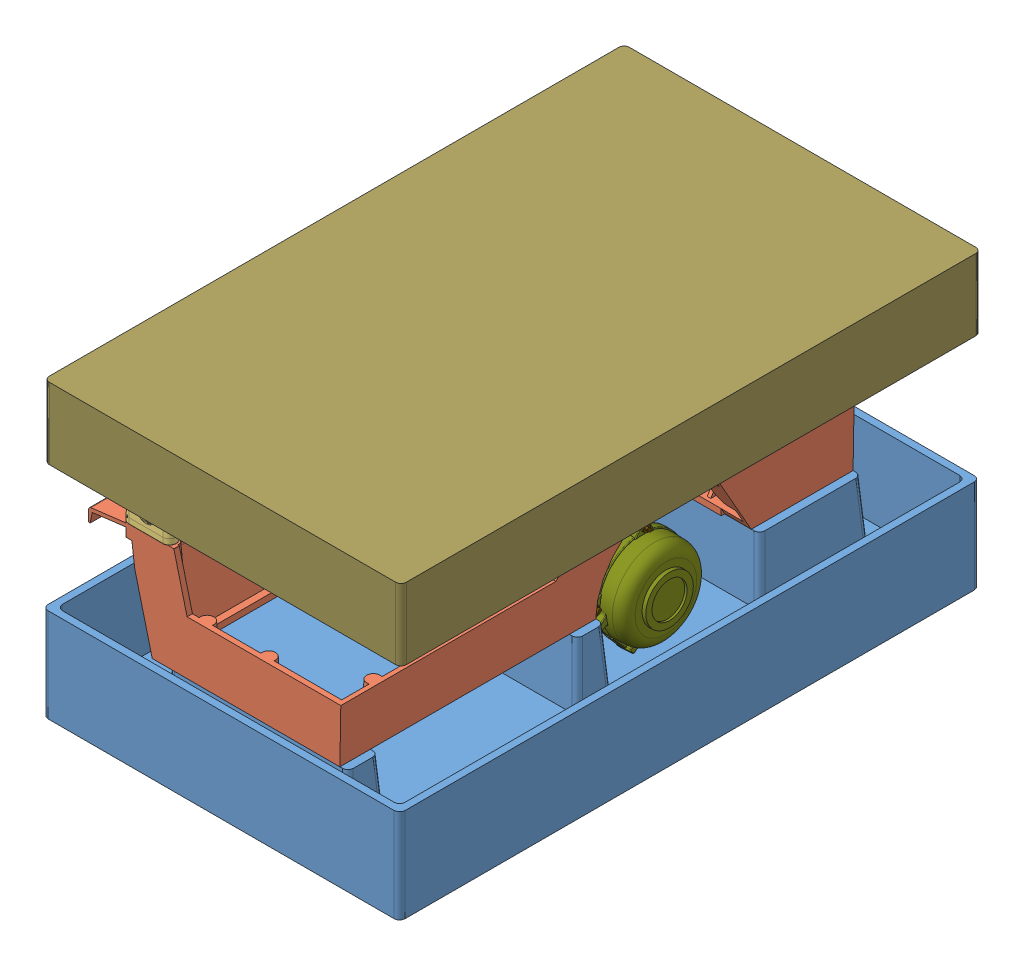
SolidWorks assembly Siège de dentiste, configuration Défaut. Lengths in mm.
Overall size (401 374.1 650.58).
134 component instances, 46 part files, 15 mates.
Components (placement in the parent):
- Chassis-1: Chassis [Défaut] at origin size (400 245.59 650)
  - Base-2: Base [Défaut] at (19.488 0 0) x (1 0 0) z (0 -1 0) size (400 650 105)
  - Chassis-1: Chassis [Défaut] at origin size (284.75 158.03 576.08)
  - Demi-bride-1: Demi-bride [Défaut] at (-215.8786 159.586 270) x (1 0 0) z (0 -1 0) size (53 15 19.91)
  - Demi-bride-2: Demi-bride [Défaut] at (-215.8786 159.586 524) x (-1 0 0) z (0 -1 0) size (53 15 19.91)
  - Demi-bride-3: Demi-bride [Défaut] at (-215.8786 118.686 524) x (1 0 0) z (0 1 0) size (53 15 19.91)
  - Demi-bride-4: Demi-bride [Défaut] at (-215.8786 118.686 270) x (-1 0 0) z (0 1 0) size (53 15 19.91)
  - Axe de guidage-1: Axe de guidage [Défaut] at (-215.8786 139.136 527.5) x (0.966925 -0.255061 0) z (0 0 -1) size (25 25 263)
  - Rondelle plate 5,3-10-1: Rondelle plate 5,3-10 [Défaut] at (-234.8786 160.586 270) x (0 -1 0) z (0 0 1) size (1 10 10)
  - Vis chc M5-50-1: Vis chc M5-50 [Défaut] at (-234.8786 160.586 270) x (0 -1 0) z (0.008588 0 0.999963) size (55 8.5 8.5)
  - Rondelle plate 5,3-10-2: Rondelle plate 5,3-10 [Défaut] at (-234.8786 160.586 524) x (0 -1 0) z (0 0 1) size (1 10 10)
  - Rondelle plate 5,3-10-3: Rondelle plate 5,3-10 [Défaut] at (-194.8786 160.586 270) x (0 -1 0) z (0 0 1) size (1 10 10)
  - Rondelle plate 5,3-10-4: Rondelle plate 5,3-10 [Défaut] at (-194.8786 160.586 524) x (0 -1 0) z (0 0 1) size (1 10 10)
  - Vis chc M5-50-2: Vis chc M5-50 [Défaut] at (-234.8786 160.586 524) x (0 -1 0) z (0.008588 0 0.999963) size (55 8.5 8.5)
  - Vis chc M5-50-3: Vis chc M5-50 [Défaut] at (-194.8786 160.586 270) x (0 -1 0) z (0.008588 0 0.999963) size (55 8.5 8.5)
  - Vis chc M5-50-4: Vis chc M5-50 [Défaut] at (-194.8786 160.586 524) x (0 -1 0) z (0.008588 0 0.999963) size (55 8.5 8.5)
  - axe 12-36 + gorge-1: axe 12-36 + gorge [Défaut] at (5.6 139.1359 -27) size (36 12 12)
  - Circlips 9-12-1: Circlips 9-12 [Défaut] at (4.1 145.1123 -27) x (0 0 1) z (-1 0 0) size (18.8 15.36 1.1)
  - Vis chc M8-20-1: Vis chc M8-20 [Défaut] at (-177.2905 7.85 55) x (0 -1 0) z (-0.152618 0 0.988285) size (28 13 13)
  - Rondelle à dent extérieure type A D8-1: Rondelle à dent extérieure type A D8 [Défaut] at (-177.2905 7.85 55) x (0 -1 0) z (0 0 1) size (0.85 15.2 15.2)
  - Vis chc M8-20-2: Vis chc M8-20 [Défaut] at (-177.2905 7.85 252) x (0 -1 0) z (-0.152618 0 0.988285) size (28 13 13)
  - Vis chc M8-20-3: Vis chc M8-20 [Défaut] at (-22.2905 7.85 55) x (0 -1 0) z (-0.152618 0 0.988285) size (28 13 13)
  - Vis chc M8-20-4: Vis chc M8-20 [Défaut] at (-22.2905 7.85 252) x (0 -1 0) z (-0.152618 0 0.988285) size (28 13 13)
  - Rondelle à dent extérieure type A D8-2: Rondelle à dent extérieure type A D8 [Défaut] at (-177.2905 7.85 252) x (0 -1 0) z (0 0 1) size (0.85 15.2 15.2)
  - Rondelle à dent extérieure type A D8-3: Rondelle à dent extérieure type A D8 [Défaut] at (-22.2905 7.85 55) x (0 -1 0) z (0 0 1) size (0.85 15.2 15.2)
  - Rondelle à dent extérieure type A D8-4: Rondelle à dent extérieure type A D8 [Défaut] at (-22.2905 7.85 252) x (0 -1 0) z (0 0 1) size (0.85 15.2 15.2)
  - Vis chc M8-20-5: Vis chc M8-20 [Défaut] at (-177.2905 7.85 505) x (0 -1 0) z (-0.152618 0 0.988285) size (28 13 13)
  - Vis chc M8-20-6: Vis chc M8-20 [Défaut] at (-23.2905 7.85 505) x (0 -1 0) z (-0.152618 0 0.988285) size (28 13 13)
  - Rondelle à dent extérieure type A D8-5: Rondelle à dent extérieure type A D8 [Défaut] at (-177.2905 7.85 505) x (0 -1 0) z (0 0 1) size (0.85 15.2 15.2)
  - Rondelle à dent extérieure type A D8-6: Rondelle à dent extérieure type A D8 [Défaut] at (-23.2905 7.85 505) x (0 -1 0) z (0 0 1) size (0.85 15.2 15.2)
  - Rondelle à dent extérieure type A D8-7: Rondelle à dent extérieure type A D8 [Défaut] at (-177.2905 12 -35) x (0 1 0) z (0 0 1) size (0.85 15.2 15.2)
  - Vis chc M8-20-7: Vis chc M8-20 [Défaut] at (-177.2905 12.85 -35) x (0 -1 0) z (0.924225 0 -0.381849) size (28 13 13)
  - Vis chc M8-20-8: Vis chc M8-20 [Défaut] at (-23.2905 12.85 -35) x (0 -1 0) z (0.924225 0 -0.381849) size (28 13 13)
  - Rondelle à dent extérieure type A D8-8: Rondelle à dent extérieure type A D8 [Défaut] at (-23.2905 12 -35) x (0 1 0) z (0 0 1) size (0.85 15.2 15.2)
  - Axe fixation moteur-1: Axe fixation moteur [Défaut] at (-187.5788 -55 97.6638) x (-1 0 0) z (0 -0.767104 -0.641522) size (65 13 13)
- Plateau-1: Plateau [Défaut] at (-53.1028 206.8102 271.423) x (-1 0 0) z (0 1 0) size (400 650 86.22)
  - Plateau supérieur-1: Plateau supérieur [Défaut] at origin size (400 650 80)
  - Demi-bride-1: Demi-bride [Défaut] at (0 0 0.686) x (-1 0 0) z (0 0 -1) size (53 15 19.91)
  - Demi-bride-2: Demi-bride [Défaut] at (0 0 -40.214) x (1 0 0) z (0 0 1) size (53 15 19.91)
  - Axe de guidage-1: Axe de guidage [Défaut] at (0 -5.5 -19.764) x (0.920339 0 0.391122) z (0 1 0) size (25 25 263)
  - Rondelle plate 5,3-10-1: Rondelle plate 5,3-10 [Défaut] at (19 0 -41.214) x (0 0 1) z (-1 0 0) size (1 10 10)
  - Vis chc M5-50-1: Vis chc M5-50 [Défaut] at (19 0 -41.214) x (0 0 1) z (0.217912 -0.975968 0) size (55 8.5 8.5)
  - Vis chc M5-50-2: Vis chc M5-50 [Défaut] at (-19 0 -41.214) x (0 0 1) z (0.217912 -0.975968 0) size (55 8.5 8.5)
  - Rondelle plate 5,3-10-2: Rondelle plate 5,3-10 [Défaut] at (-19 0 -41.214) x (0 0 1) z (-1 0 0) size (1 10 10)
  - Demi-bride-3: Demi-bride [Défaut] at (-0.8646 254.5 0.6677) x (0.999106 0 0.042279) z (0.042279 0 -0.999106) size (53 15 19.91)
  - Demi-bride-4: Demi-bride [Défaut] at (0.8646 254.5 -40.1957) x (-0.999106 0 -0.042279) z (-0.042279 0 0.999106) size (53 15 19.91)
  - Rondelle plate 5,3-10-3: Rondelle plate 5,3-10 [Défaut] at (19 254 -41.214) x (0 0 1) z (-1 0 0) size (1 10 10)
  - Rondelle plate 5,3-10-4: Rondelle plate 5,3-10 [Défaut] at (-19 254 -41.214) x (0 0 1) z (-1 0 0) size (1 10 10)
  - Vis chc M5-50-3: Vis chc M5-50 [Défaut] at (19 254 -41.214) x (0 0 1) z (0.217912 -0.975968 0) size (55 8.5 8.5)
  - Vis chc M5-50-4: Vis chc M5-50 [Défaut] at (-19 254 -41.214) x (0 0 1) z (0.217912 -0.975968 0) size (55 8.5 8.5)
  - axe 12-36 + gorge-1: axe 12-36 + gorge [Défaut] at (222.5997 -298.148 -19.7641) x (1 0 0) z (0 0.681003 0.732281) size (36 12 12)
  - Circlips 9-12-1: Circlips 9-12 [Défaut] at (221.0997 -292.1717 -19.7641) x (0 0 1) z (-1 0 0) size (18.8 15.36 1.1)
  - Ecrou H M12-1: Ecrou H M12 [Défaut] at (19.4997 -298.423 -19.7641) x (1 0 0) z (0 0 -1) size (6 20.78 18)
  - Ecrou H M12-2: Ecrou H M12 [Défaut] at (25.4997 -298.423 -19.7641) x (1 0 0) z (0 0 -1) size (6 20.78 18)
- Ciseau A-1: Ciseau A [Défaut] at (-254.6024 205.9809 218.8502) x (0 0.092135 -0.995747) z (-1 0 0) size (555.5 69.46 246.27)
  - Ciseau A-1: Ciseau A [Défaut] at (243.06 41.5056 0) size (555 69.46 239.27)
  - coussinet d16_15-1: coussinet d16_15 [Défaut] at (-16.94 41.5056 -217.5) x (0.656107 -0.754667 0) z (0 0 1) size (18 18 15)
  - coussinet d12_10-1: coussinet d12_10 [Défaut] at (243.06 41.5056 6.5) size (14 14 10)
  - Coussinet épaulé-2: Coussinet épaulé [Défaut] at (243.06 41.5056 -215.5) x (0 0 1) z (-1 0 0) size (11.59 19.86 20)
  - Axe 16_93-1: Axe 16_93 [Défaut] at (-16.94 41.5056 11) x (0 0 1) z (-0.999233 0.039166 0) size (93 16 16)
  - Circlips 15-1-1: Circlips 15-1 [Défaut] at (-16.94 49.5056 -79.5) size (19.3 20.94 1)
  - Circlips 15-1-2: Circlips 15-1 [Défaut] at (-23.7604 45.6869 7.5) x (0.522659 0.852542 0) z (0 0 1) size (19.3 20.94 1)
  - Ecrou H M16-1: Ecrou H M16 [Défaut] at (-276.94 41.5056 13.5) x (0 0 -1) z (1 0 0) size (8 27.71 24)
  - Ecrou H M16-2: Ecrou H M16 [Défaut] at (-276.94 41.5056 -91.5) x (0 0 1) z (-1 0 0) size (8 27.71 24)
  - Rondelle 15-36-2-1: Rondelle 15-36-2 [Défaut] at (243.06 41.5056 -224.5) size (36 36 2)
  - Vis axe H M12-55-1: Vis axe H M12-55 [Défaut] at (243.06 41.5056 -224.5) x (-0.923728 -0.383049 0) z (0 0 -1) size (27.71 24 60)
- Ciseau B-1: Ciseau B [Défaut] at (-14.1024 128.9526 166.2652) x (0 -0.092135 -0.995747) z (1 0 0) size (561.02 117.93 246.2)
  - Ciseau B-1: Ciseau B [Défaut] at (191.5049 27.9465 0) size (555 113.04 239.2)
  - coussinet d12_10-1: coussinet d12_10 [Défaut] at (191.5049 27.9465 6.5) x (0.99814 -0.060957 0) z (0 0 1) size (14 14 10)
  - coussinet d16_15-1: coussinet d16_15 [Défaut] at (-68.4951 27.9465 -217.5) size (18 18 15)
  - Coussinet épaulé-1: Coussinet épaulé [Défaut] at (191.5049 27.9465 -215.5) x (0 0 1) z (-0.532611 0.84636 0) size (11.59 19.86 20)
  - Ecrou H M16-1: Ecrou H M16 [Défaut] at (-54.4951 -46.5535 -198) x (0 0 1) z (-0.996809 0.079821 0) size (8 27.71 24)
  - Ecrou H M16-2: Ecrou H M16 [Défaut] at (-54.4951 -46.5535 -89.5) x (0 0 1) z (-0.59499 0.803733 0) size (8 27.71 24)
  - Ecrou H M16-3: Ecrou H M16 [Défaut] at (-328.4951 27.9465 -91.5) x (0 0 1) z (-1 0 0) size (8 27.71 24)
  - Ecrou H M16-4: Ecrou H M16 [Défaut] at (-328.4951 27.9465 5.5) x (0 0 1) z (-1 0 0) size (8 27.71 24)
  - Axe 16_93-1: Axe 16_93 [Défaut] at (-68.4951 27.9465 11) x (0 0 1) z (-0.710378 0.70382 0) size (93 16 16)
  - Circlips 15-1-1: Circlips 15-1 [Défaut] at (-68.4355 35.9463 7.5) x (0.999972 -0.00745 0) z (0 0 1) size (19.3 20.94 1)
  - Circlips 15-1-2: Circlips 15-1 [Défaut] at (-68.4951 35.9465 -79.5) size (19.3 20.94 1)
  - Ecrou H M12-1: Ecrou H M12 [Défaut] at (191.5049 27.9465 -177.5) x (0 0 -1) z (0.286555 0.958064 0) size (6 20.78 18)
  - Ecrou H M12-2: Ecrou H M12 [Défaut] at (191.5049 27.9465 -171.5) x (0 0 -1) z (0.286555 0.958064 0) size (6 20.78 18)
  - Rondelle 15-36-2-1: Rondelle 15-36-2 [Défaut] at (191.5049 27.9465 -222.5) x (-0.923728 -0.383049 0) z (0 0 -1) size (36 36 2)
  - Vis axe H M12-55-1: Vis axe H M12-55 [Défaut] at (191.5049 27.9465 -224.5) x (-0.923728 -0.383049 0) z (0 0 -1) size (27.71 24 60)
- Palier guide-1: Palier guide [Défaut] at (-215.8786 139.136 490.7882) x (0 0 1) z (-1 0 0) size (32 50 102)
  - Palier guide-1: Palier guide [Défaut] at origin size (32 50 52)
  - Coussinet épaulé-1: Coussinet épaulé [Défaut] at (0 0 15.5) x (0 0 1) z (-1 0 0) size (11.59 19.86 20)
  - Coussinet épaulé-2: Coussinet épaulé [Défaut] at (0 0 -15.5) x (0 0 -1) z (1 0 0) size (11.59 19.86 20)
  - coussinet d25_40-2: coussinet d25_40 [Défaut] at (-16 0 0) size (32 28 28)
  - Vis sans tête fendue téton long-1: Vis sans tête fendue téton long [Défaut] at (0 0 45.7338) x (0 0 -1) z (1 0 0) size (35 16 16)
  - Vis sans tête fendue téton long-2: Vis sans tête fendue téton long [Défaut] at (0 0 -45.7338) x (0 0 1) z (-1 0 0) size (35 16 16)
- Palier guide-2: Palier guide [Défaut] at (-53.1028 187.0462 490.7882) x (0 0 1) z (1 0 0) size (32 50 102)
  - Palier guide-1: Palier guide [Défaut] at origin size (32 50 52)
  - Coussinet épaulé-1: Coussinet épaulé [Défaut] at (0 0 15.5) x (0 0 1) z (-1 0 0) size (11.59 19.86 20)
  - Coussinet épaulé-2: Coussinet épaulé [Défaut] at (0 0 -15.5) x (0 0 -1) z (1 0 0) size (11.59 19.86 20)
  - coussinet d25_40-2: coussinet d25_40 [Défaut] at (-16 0 0) size (32 28 28)
  - Vis sans tête fendue téton long-1: Vis sans tête fendue téton long [Défaut] at (0 0 45.7338) x (0 0 -1) z (1 0 0) size (35 16 16)
  - Vis sans tête fendue téton long-2: Vis sans tête fendue téton long [Défaut] at (0 0 -45.7338) x (0 0 1) z (-1 0 0) size (35 16 16)
- Porte Ecrou-1: Porte Ecrou [Défaut] at (-149.2539 92.6129 229.2229) x (0 0.749988 0.661451) z (0 -0.661451 0.749988) size (42.3 120 81.63)
  - Porte écrou-1: Porte écrou [Défaut] at (10.3401 26.4221 0) size (35.51 70 81.63)
  - Coussinet épaulé-1: Coussinet épaulé [Défaut] at (-6.6599 -17.8279 0) x (0 -1 0) z (0.664763 0 0.747055) size (11.59 19.86 20)
  - Coussinet épaulé-2: Coussinet épaulé [Défaut] at (-6.6599 31.1721 0) x (0 1 0) z (0 0 1) size (11.59 19.86 20)
  - Ecrou-1: Ecrou [Défaut] at (10.8401 6.6721 0) x (1 0 0) z (0 -0.057243 -0.99836) size (40.8 44 44)
  - Bride ecrou-1: Bride ecrou [Défaut] at (-14.6599 26.4221 0) size (6 61.5 61.5)
  - local.ISO.14.35-1: local.ISO.14.35 [Défaut] at (-20.6599 6.6721 -26.6806) x (1 0 0) z (0 0.781637 0.623734) size (12.82 6.12 6.4)
  - local.ISO.14.35-2: local.ISO.14.35 [Défaut] at (-20.6599 -16.434 13.3403) x (1 0 0) z (0 0.149351 -0.988784) size (12.82 6.12 6.4)
  - local.ISO.14.35-3: local.ISO.14.35 [Défaut] at (-20.6599 29.7781 13.3403) x (1 0 0) z (0 -0.930988 0.365051) size (12.82 6.12 6.4)
  - Vis sans tête fendue téton long-1: Vis sans tête fendue téton long [Défaut] at (-6.6599 61.4059 0) x (0 -1 0) z (-0.111323 0 0.993784) size (35 16 16)
  - Vis sans tête fendue téton long-2: Vis sans tête fendue téton long [Défaut] at (-6.6599 -48.0618 0) x (0 1 0) z (-0.099587 0 0.995029) size (35 16 16)
- Motoréducteur-1: Motoréducteur [Défaut] at (-116.0264 -5.1242 179.5234) x (0.999948 0.006774 -0.007681) z (0.010241 -0.661417 0.749949) size (201.23 154.73 109.91)
  - Carter Réducteur-1: Carter Réducteur [Défaut] at (5.8828 -7.0876 0) size (100.4 99.45 106.51)
  - chape fixation moteur sdd-1: chape fixation moteur sdd [Défaut] at (-39.6129 -81.9915 -28.4584) x (0 1 0) z (-0.99998 0 -0.006259) size (60 54 54)
  - couvercle réducteur sdd-1: couvercle réducteur sdd [Défaut] at (-67.1172 -24.3796 -30.4416) x (0 0 1) z (1 0 0) size (82.77 82.77 11.01)
  - Flasque arrière-1: Flasque arrière [Défaut] at (69.9422 -7.0876 0) size (40 99.43 99.43)
  - stator-1: stator [Défaut] at (66.5828 -7.0876 0) x (-1 0 0) z (0 -0.007925 -0.999969) size (91.4 91.92 91.92)
  - tirant d'assemblage moteur sdd-1: tirant d'assemblage moteur sdd [Défaut] at (14.4988 5.6366 38.1838) x (0 1 0) z (0 0 1) size (8 99 8)
  - tirant d'assemblage moteur sdd-2: tirant d'assemblage moteur sdd [Défaut] at (14.4988 -45.2714 12.7242) x (0 0 1) z (0 -1 0) size (8 99 8)
  - tirant d'assemblage moteur sdd-3: tirant d'assemblage moteur sdd [Défaut] at (14.4988 -19.8118 -38.1838) x (0 -1 0) z (0 0 -1) size (8 99 8)
  - tirant d'assemblage moteur sdd-4: tirant d'assemblage moteur sdd [Défaut] at (14.4988 31.0961 -12.7242) x (0 0 -1) z (0 1 0) size (8 99 8)
  - plaque de serrage bis-1: plaque de serrage bis [Défaut] at (-39.7017 32.9196 -14.2817) x (-0.006259 0 0.99998) z (0 1 0) size (85 74 5)
  - plaque deserrage-1: plaque deserrage [Défaut] at (-39.7017 -52.0949 -14.2817) x (-0.006259 0 0.99998) z (0 1 0) size (85 74 5)
  - tirant d'assemblage sdd-1: tirant d'assemblage sdd [Défaut] at (-13.9904 32.6891 17.0675) size (10 98 10)
  - tirant d'assemblage sdd-2: tirant d'assemblage sdd [Défaut] at (-13.5585 32.6891 -51.9312) size (10 98 10)
  - tirant d'assemblage sdd-3: tirant d'assemblage sdd [Défaut] at (-56.4873 32.6891 -29.5329) x (-0.99923 0 -0.039233) z (0.039233 0 -0.99923) size (10 98 10)
  - vis_uni_6109_-_m5-_0_8-_16-1: vis_uni_6109_-_m5-_0_8-_16 [Défaut] at (-61.1172 26.9124 18.7186) x (0 0.002509 0.999997) z (1 0 0) size (9.2 9.12 16)
  - vis_uni_6109_-_m5-_0_8-_16-2: vis_uni_6109_-_m5-_0_8-_16 [Défaut] at (-60.6916 26.9124 -49.2801) x (0 0.002509 0.999997) z (1 0 0) size (9.2 9.12 16)
  - vis_uni_6109_-_m5-_0_8-_16-3: vis_uni_6109_-_m5-_0_8-_16 [Défaut] at (-61.1172 -41.0876 18.7186) x (0 0.002509 0.999997) z (1 0 0) size (9.2 9.12 16)
  - vis_uni_6109_-_m5-_0_8-_16-4: vis_uni_6109_-_m5-_0_8-_16 [Défaut] at (-60.6916 -41.0876 -49.2801) x (0 0.002509 0.999997) z (1 0 0) size (9.2 9.12 16)
  - goupille_elastique_nf_e_27-489_5x10-1: goupille_elastique_nf_e_27-489_5x10 [Défaut] at (-55.6263 -50.0949 -11.9714) x (0.874297 0 0.485391) z (0 -1 0) size (4.99 5 10)
  - goupille_elastique_nf_e_27-489_5x10-2: goupille_elastique_nf_e_27-489_5x10 [Défaut] at (-23.608 -50.0949 -43.5914) x (-0.874297 0 -0.485391) z (0 -1 0) size (4.99 5 10)
  - bague de mise en position-1: bague de mise en position [Défaut] at (-45.0735 -47.0949 -31.8697) x (-0.837169 0 -0.546944) z (0 1 0) size (33 33 22)
- Vis-1: Vis [Défaut] at (-164.5854 77.5411 237.0191) x (0 -0.749988 -0.661451) z (0.877142 -0.317649 0.360168) size (355 47.55 47.55)
  - vis de sortie motored sdd-1: vis de sortie motored sdd [Défaut] at (-138.3393 10.6027 0) size (344 20 20)
  - butée de déplacement coté moteur-1: butée de déplacement coté moteur [Défaut] at (48.5057 23.0038 -0.1139) x (1 0 0) z (0 0.022895 0.999738) size (20 46.5 46.5)
  - butée de déplacement coté vis-1: butée de déplacement coté vis [Défaut] at (-189.6494 18.0155 0.3226) x (-1 0 0) z (0 -0.998753 -0.049934) size (11 24 24)
  - vis_fhc_nf_e_27-160_m10x1_5-25-1: vis_fhc_nf_e_27-160_m10x1_5-25 [Défaut] at (-189.391 18.0316 0) x (0 0.586298 0.810096) z (-1 0 0) size (18.3 18.3 25)
Mates (geometry in assembly coordinates):
- Coïncidente22: coincident: point of Chassis-1/Chassis-1; point of Motoréducteur-1
- Coaxiale35: concentric: cylinder of Chassis-1/Axe de guidage-1 through (-215.8786 139.136 527.5) axis (0 0 -1) radius 12.5; cylinder of Palier guide-1/coussinet d25_40-2 through (-215.8786 139.136 474.7882) axis (0 0 -1) radius 12.5
- Coaxiale37: concentric: cylinder of Plateau-1/Axe de guidage-1 through (-53.1028 187.0462 265.923) axis (0 0 1) radius 12.5; cylinder of Palier guide-2/coussinet d25_40-2 through (-53.1028 187.0462 474.7882) axis (0 0 -1) radius 12.5
- Coaxiale45: concentric: cylinder of Chassis-1/axe 12-36 + gorge-1 through (-13.75 139.1359 -27) axis (1 0 0) radius 6; cylinder of Ciseau B-1/coussinet d12_10-1 through (-7.6024 139.1359 -27) axis (-1 0 0) radius 6
- Coaxiale46: concentric: cylinder of Ciseau B-1/Ciseau B-1 through (410.461 87.6181 224.8177) axis (-1 0 0) radius 7.188; cylinder of Porte Ecrou-1/Vis sans tête fendue téton long-2 through (-107.926 87.6181 224.8177) axis (-1 0 0) radius 8
- Coaxiale47: concentric: cylinder of Ciseau B-1/Ciseau B-1 through (-85.6024 187.0462 490.7882) axis (-1 0 0) radius 7; cylinder of Palier guide-2/Vis sans tête fendue téton long-2 through (-92.1028 187.0462 490.7882) axis (1 0 0) radius 8
- Coaxiale48: concentric: cylinder of Ciseau A-1/coussinet d16_15-1 through (-37.1024 163.0911 231.8941) axis (1 0 0) radius 8; cylinder of Ciseau B-1/Axe 16_93-1 through (-49.6024 163.0911 231.8941) axis (1 0 0) radius 8
- Coaxiale49: concentric: cylinder of Ciseau A-1/Ecrou H M16-2 through (-133.3556 139.136 490.7882) axis (-1 0 0) radius 6.9175; cylinder of Palier guide-1/Vis sans tête fendue téton long-2 through (-176.8786 139.136 490.7882) axis (-1 0 0) radius 8
- Coïncidente23: coincident: plane of Chassis-1/Chassis-1 through (-7.6024 71.835 -20.1314) normal (-1 0 0); plane of Ciseau B-1/Ciseau B-1 through (-7.6024 139.1359 -27) normal (1 0 0)
- Coïncidente24: coincident: plane of Ciseau A-1/Ciseau A-1 through (-22.1024 163.0911 231.8941) normal (1 0 0); plane of Ciseau B-1/Ciseau B-1 through (-22.1024 142.696 233.7812) normal (-1 0 0)
- Coaxiale50: concentric: cylinder of Plateau-1/Plateau supérieur-1 through (-50.6024 187.0461 -27) axis (-1 0 0) radius 6; cylinder of Ciseau A-1/Vis axe H M12-55-1 through (-30.1024 187.0461 -27) axis (-1 0 0) radius 6
- Coïncidente26: coincident: plane of Plateau-1/Plateau supérieur-1 through (-50.6024 209.6804 -33.5103) normal (1 0 0); plane of Ciseau A-1/Coussinet épaulé-2 through (-50.6024 177.1269 -28.2683) normal (-1 0 0)
- Coaxiale52: concentric: cylinder of Porte Ecrou-1/Ecrou-1 through (-155.926 125.9489 258.6236) axis (0 -0.749988 -0.661451) radius 8; cylinder of Vis-1/vis de sortie motored sdd-1 through (-155.926 140.4202 271.3865) axis (0 -0.749988 -0.661451) radius 10
- Coaxiale53: concentric: cylinder of Vis-1/vis de sortie motored sdd-1 through (-155.926 17.0472 162.5778) axis (0 -0.749988 -0.661451) radius 7.5; cylinder of Motoréducteur-1/chape fixation moteur sdd-1 through (-155.926 -57.2125 97.0846) axis (0 0.749988 0.661451) radius 19
- Distance3: distance = 17.5 mm: plane of Vis-1/butée de déplacement coté moteur-1 through (-147.5881 65.1915 183.5806) normal (0 -0.749988 -0.661451); plane of Motoréducteur-1/plaque de serrage bis-1 through (-156.3372 36.9202 189.1791) normal (0 0.749988 0.661451)
